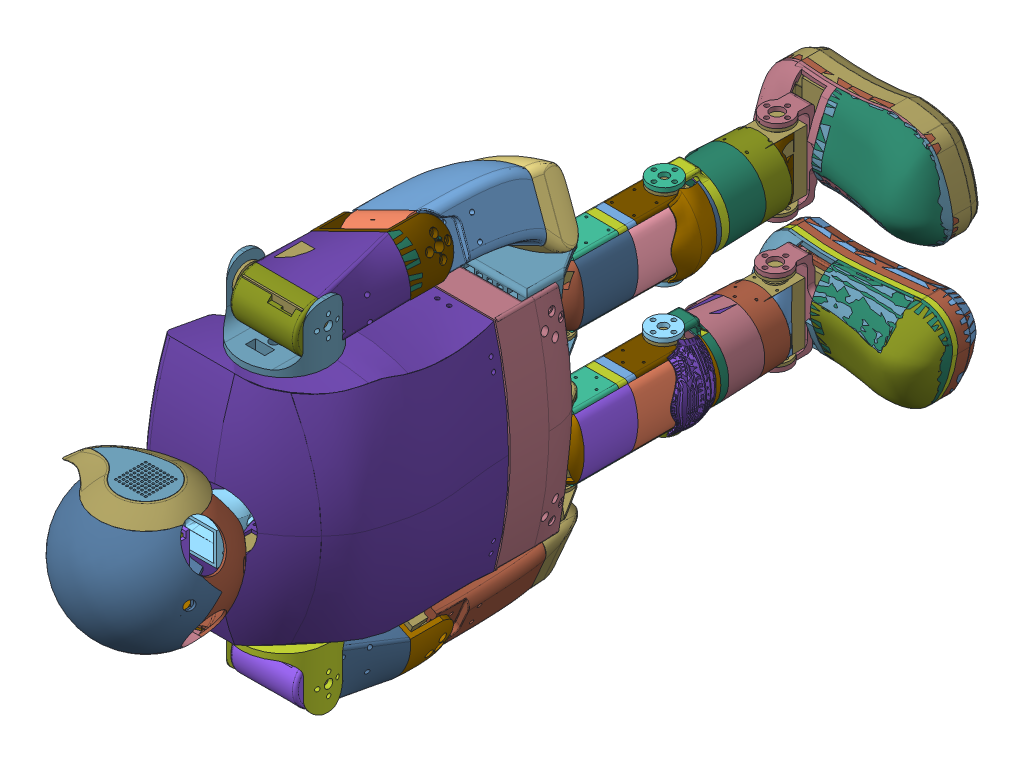
SolidWorks assembly ROBOT, configuration Default. Lengths in mm.
Overall size (168.02 284.66 497.18).
184 component instances, 104 part files, 132 mates.
Components (placement in the parent):
- right foot-1: right foot [Default] at (47.4769 97.6627 319.5854) size (123.36 70.36 23.98)
  - right foot-Part-1-1: right foot-Part-1 [默认] at (2.4797 75.1958 -228.2622) x (0 -1 0) z (0 0 1) size (70.36 123.36 10.26)
  - right foot-Part-2-1: right foot-Part-2 [默认] at (2.4797 75.1958 -228.2622) x (0 -1 0) z (0 0 1) size (5 5 3)
  - right foot-Part-3-1: right foot-Part-3 [默认] at (2.4797 75.1958 -228.2622) x (0 -1 0) z (0 0 1) size (5 5 3)
  - right foot-Part-4-1: right foot-Part-4 [默认] at (2.4797 75.1958 -228.2622) x (0 -1 0) z (0 0 1) size (5 5 3)
  - right foot-Part-5-1: right foot-Part-5 [默认] at (2.4797 75.1958 -228.2622) x (0 -1 0) z (0 0 1) size (3 3 3)
  - right foot-Part-6-1: right foot-Part-6 [默认] at (2.4797 75.1958 -228.2622) x (0 -1 0) z (0 0 1) size (3 3 3)
  - right foot-Part-7-1: right foot-Part-7 [默认] at (2.4797 75.1958 -228.2622) x (0 -1 0) z (0 0 1) size (68.42 123.23 13.95)
  - right foot-Part-8-1: right foot-Part-8 [默认] at (2.4797 75.1958 -228.2622) x (0 -1 0) z (0 0 1) size (3 3 3)
  - right foot-Part-9-1: right foot-Part-9 [默认] at (2.4797 75.1958 -228.2622) x (0 -1 0) z (0 0 1) size (5 5 3)
  - right foot-Part-10-1: right foot-Part-10 [默认] at (2.4797 75.1958 -228.2622) x (0 -1 0) z (0 0 1) size (3 3 3)
  - right foot-Part-11-1: right foot-Part-11 [默认] at (2.4797 75.1958 -228.2622) x (0 -1 0) z (0 0 1) size (70.36 123.36 19.01)
- servo-1: servo [Default] at (64.0611 111.5585 116.4732) x (0 0 1) z (0 1 0) size (20 51.7 40)
  - servo-Part-1-1: servo-Part-1 [默认] at (-33.15 -9.3942 -72.6) x (0 0 1) z (1 0 0) size (40 51.7 20)
- zhijiao-1: zhijiao [Default] at (47.3569 97.6627 319.5854) size (59.38 57.38 56.66)
  - zhijiao-Part-1-1: zhijiao-Part-1 [默认] at (-38.15 -124.7042 -221.2622) x (0 -1 0) z (-1 0 0) size (57.38 56.66 59.38)
- right foot cover-1: right foot cover [Default] at (47.5769 97.6627 319.5854) size (124.44 71 32.97)
  - right foot cover-Part-1-1: right foot cover-Part-1 [默认] at (2.3797 137.8816 -227.2622) x (0 -1 0) z (0 0 1) size (71 123.7 31.71)
  - right foot cover-Part-2-1: right foot cover-Part-2 [默认] at (2.3797 137.8816 -227.2622) x (0 -1 0) z (0 0 1) size (65.9 77.18 26.11)
  - right foot cover-Part-3-1: right foot cover-Part-3 [默认] at (2.3797 137.8816 -227.2622) x (0 -1 0) z (0 0 1) size (65.83 76.7 26.08)
- servo-2: servo [Default] at (1.0324 97.7127 87.3987) x (-1 0 0.000575) z (-0.000575 0 -1) size (20 51.7 40)
  - servo-Part-1-1: servo-Part-1 [默认] at (-33.15 -9.3942 -72.6) x (0 0 1) z (1 0 0) size (40 51.7 20)
- shank right-1: shank right [Default] at (14.2241 -102.1815 159.9911) x (-0.000575 0 -1) z (1 0 -0.000575) size (92.37 57.6 51.33)
  - shank right-Part-1-1: shank right-Part-1 [默认] at origin size (25 48.39 47.26)
  - shank right-Part-2-1: shank right-Part-2 [默认] at origin size (18.05 46 46)
  - shank right-Part-3-1: shank right-Part-3 [默认] at origin size (23.16 40.51 12.38)
  - shank right-Part-4-1: shank right-Part-4 [默认] at origin size (3 2.5 26)
  - shank right-Part-5-1: shank right-Part-5 [默认] at origin size (3 2.5 26)
  - shank right-Part-6-1: shank right-Part-6 [默认] at origin size (3 2.5 26)
  - shank right-Part-7-1: shank right-Part-7 [默认] at origin size (20 2.9 20)
  - shank right-Part-8-1: shank right-Part-8 [默认] at origin size (20 2.9 20)
  - shank right-Part-9-1: shank right-Part-9 [默认] at origin size (14.44 57.6 31.5)
  - shank right-Part-10-1: shank right-Part-10 [默认] at origin size (31.11 53.53 20.13)
  - shank right-Part-11-1: shank right-Part-11 [默认] at origin size (5.05 44.63 15.49)
  - shank right-Part-12-1: shank right-Part-12 [默认] at origin size (23.29 40.51 12.38)
  - shank right-Part-13-1: shank right-Part-13 [默认] at origin size (18.05 46 46)
  - shank right-Part-14-1: shank right-Part-14 [默认] at origin size (3 2.5 26)
  - shank right-Part-15-1: shank right-Part-15 [默认] at origin size (25 48.39 47.26)
  - shank right-Part-16-1: shank right-Part-16 [默认] at origin size (14.32 43.75 29.27)
  - shank right-Part-17-1: shank right-Part-17 [默认] at origin size (14.44 57.6 31.5)
  - shank right-Part-18-1: shank right-Part-18 [默认] at origin size (20 2.9 20)
  - shank right-Part-19-1: shank right-Part-19 [默认] at origin size (31.11 53.53 20.13)
- servo-3: servo [Default] at (1.1 97.6627 162.3854) x (-1 0 0) z (0 0 -1) size (20 51.7 40)
  - servo-Part-1-1: servo-Part-1 [默认] at (-33.15 -9.3942 -72.6) x (0 0 1) z (1 0 0) size (40 51.7 20)
- thigh-1: thigh [Default] at (1.1 127.7685 319.5854) x (-1 0 0) z (0 0 1) size (38.49 44.5 95.37)
  - thigh-Part-1-1: thigh-Part-1 [默认] at (-13.15 39.5 -84.6) x (0 1 0) z (0 0 1) size (44.5 24 30)
  - thigh-Part-2-1: thigh-Part-2 [默认] at (-13.15 39.5 -84.6) x (0 1 0) z (0 0 1) size (44.5 24 6)
  - thigh-Part-3-1: thigh-Part-3 [默认] at (-13.15 39.5 -84.6) x (0 1 0) z (0 0 1) size (40.5 9.43 36)
  - thigh-Part-4-1: thigh-Part-4 [默认] at (-13.15 39.5 -84.6) x (0 1 0) z (0 0 1) size (40.51 12.57 12)
  - thigh-Part-5-1: thigh-Part-5 [默认] at (-13.15 39.5 -84.6) x (0 1 0) z (0 0 1) size (40.5 9.43 36)
  - thigh-Part-6-1: thigh-Part-6 [默认] at (-13.15 39.5 -84.6) x (0 1 0) z (0 0 1) size (40.51 12.57 12.08)
  - thigh-Part-7-1: thigh-Part-7 [默认] at (-13.15 39.5 -84.6) x (0 1 0) z (0 0 1) size (44.5 24 30)
  - thigh-Part-8-1: thigh-Part-8 [默认] at (-13.15 39.5 -84.6) x (0 1 0) z (0 0 1) size (44.5 24 6)
  - thigh-Part-9-1: thigh-Part-9 [默认] at (-13.15 39.5 -84.6) x (0 1 0) z (0 0 1) size (40.5 9.43 36)
  - thigh-Part-10-1: thigh-Part-10 [默认] at (-13.15 39.5 -84.6) x (0 1 0) z (0 0 1) size (40.51 12.57 12.08)
  - thigh-Part-11-1: thigh-Part-11 [默认] at (-13.15 39.5 -84.6) x (0 1 0) z (0 0 1) size (40.5 9.43 36)
  - thigh-Part-12-1: thigh-Part-12 [默认] at (-13.15 39.5 -84.6) x (0 1 0) z (0 0 1) size (40.51 12.57 11.4)
- servo-4: servo [Default] at (47.4 97.6627 319.5854) size (20 51.7 40)
  - servo-Part-1-1: servo-Part-1 [默认] at (-33.15 -9.3942 -72.6) x (0 0 1) z (1 0 0) size (40 51.7 20)
- bottom right-1: bottom right [Default] at (47.4 97.6627 319.5854) size (44.79 57.7 52.6)
  - bottom right-Part-1-1: bottom right-Part-1 [默认] at (-42.5 42.9558 -20) size (44.79 57.7 52.6)
- servo-5: servo [Default] at (-4.4942 16.3185 332.7354) x (0 0 1) z (0 -1 0) size (20 51.7 40)
  - servo-Part-1-1: servo-Part-1 [默认] at (-33.15 -9.3942 -72.6) x (0 0 1) z (1 0 0) size (40 51.7 20)
- buttocks-1: buttocks [Default] at (47.4 97.6627 319.5854) size (72.1 145.63 51.57)
- servo-6: servo [Default] at (-4.4942 209.1127 286.4354) x (0 0 -1) z (0 1 0) size (20 51.7 40)
  - servo-Part-1-1: servo-Part-1 [默认] at (-33.15 -9.3942 -72.6) x (0 0 1) z (1 0 0) size (40 51.7 20)
- bottom left-2: bottom left [Default] at (47.4 97.6627 319.5854) size (44.75 57.7 52.6)
  - bottom left-Part-1-1: bottom left-Part-1 [默认] at (-42.5 38.85 -20) size (44.75 57.7 52.6)
- servo-8: servo [Default] at (0.7557 127.7685 319.3965) x (-0.999967 0 -0.0081) z (-0.0081 0 0.999967) size (20 51.7 40)
  - servo-Part-1-1: servo-Part-1 [默认] at (-33.15 -9.3942 -72.6) x (0 0 1) z (1 0 0) size (40 51.7 20)
- thigh-2: thigh [Default] at (47.0542 97.6627 319.7715) x (0.999967 0 0.0081) z (-0.0081 0 0.999967) size (38.49 44.5 95.37)
  - thigh-Part-1-1: thigh-Part-1 [默认] at (-13.15 39.5 -84.6) x (0 1 0) z (0 0 1) size (44.5 24 30)
  - thigh-Part-2-1: thigh-Part-2 [默认] at (-13.15 39.5 -84.6) x (0 1 0) z (0 0 1) size (44.5 24 6)
  - thigh-Part-3-1: thigh-Part-3 [默认] at (-13.15 39.5 -84.6) x (0 1 0) z (0 0 1) size (40.5 9.43 36)
  - thigh-Part-4-1: thigh-Part-4 [默认] at (-13.15 39.5 -84.6) x (0 1 0) z (0 0 1) size (40.51 12.57 12)
  - thigh-Part-5-1: thigh-Part-5 [默认] at (-13.15 39.5 -84.6) x (0 1 0) z (0 0 1) size (40.5 9.43 36)
  - thigh-Part-6-1: thigh-Part-6 [默认] at (-13.15 39.5 -84.6) x (0 1 0) z (0 0 1) size (40.51 12.57 12.08)
  - thigh-Part-7-1: thigh-Part-7 [默认] at (-13.15 39.5 -84.6) x (0 1 0) z (0 0 1) size (44.5 24 30)
  - thigh-Part-8-1: thigh-Part-8 [默认] at (-13.15 39.5 -84.6) x (0 1 0) z (0 0 1) size (44.5 24 6)
  - thigh-Part-9-1: thigh-Part-9 [默认] at (-13.15 39.5 -84.6) x (0 1 0) z (0 0 1) size (40.5 9.43 36)
  - thigh-Part-10-1: thigh-Part-10 [默认] at (-13.15 39.5 -84.6) x (0 1 0) z (0 0 1) size (40.51 12.57 12.08)
  - thigh-Part-11-1: thigh-Part-11 [默认] at (-13.15 39.5 -84.6) x (0 1 0) z (0 0 1) size (40.5 9.43 36)
  - thigh-Part-12-1: thigh-Part-12 [默认] at (-13.15 39.5 -84.6) x (0 1 0) z (0 0 1) size (40.51 12.57 11.4)
- servo-9: servo [Default] at (48.3275 127.7685 162.5766) x (0.999967 0 0.0081) z (0.0081 0 -0.999967) size (20 51.7 40)
  - servo-Part-1-1: servo-Part-1 [默认] at (-33.15 -9.3942 -72.6) x (0 0 1) z (1 0 0) size (40 51.7 20)
- shank left-1: shank left [Default] at (15.198 137.2127 159.9082) x (0.0081 0 -0.999967) z (0.999967 0 0.0081) size (92.37 57.6 51.33)
  - shank left-Part-1-1: shank left-Part-1 [默认] at origin size (25 48.39 47.26)
  - shank left-Part-2-1: shank left-Part-2 [默认] at origin size (18.05 46 46)
  - shank left-Part-3-1: shank left-Part-3 [默认] at origin size (23.29 40.51 12.38)
  - shank left-Part-4-1: shank left-Part-4 [默认] at origin size (23.16 40.51 12.38)
  - shank left-Part-5-1: shank left-Part-5 [默认] at origin size (3 2.5 26)
  - shank left-Part-6-1: shank left-Part-6 [默认] at origin size (3 2.5 26)
  - shank left-Part-7-1: shank left-Part-7 [默认] at origin size (3 2.5 26)
  - shank left-Part-8-1: shank left-Part-8 [默认] at origin size (3 2.5 26)
  - shank left-Part-9-1: shank left-Part-9 [默认] at origin size (20 2.9 20)
  - shank left-Part-10-1: shank left-Part-10 [默认] at origin size (20 2.9 20)
  - shank left-Part-11-1: shank left-Part-11 [默认] at origin size (14.44 57.6 31.5)
  - shank left-Part-12-1: shank left-Part-12 [默认] at origin size (14.32 43.75 29.27)
  - shank left-Part-13-1: shank left-Part-13 [默认] at origin size (31.11 53.53 20.13)
  - shank left-Part-14-1: shank left-Part-14 [默认] at origin size (5.05 44.63 15.49)
- servo-10: servo [Default] at (48.935 127.8185 87.5791) x (0.999967 0 0.0081) z (0.0081 0 -0.999967) size (20 51.7 40)
  - servo-Part-1-1: servo-Part-1 [默认] at (-33.15 -9.3942 -72.6) x (0 0 1) z (1 0 0) size (40 51.7 20)
- zhijiao-2: zhijiao [Default] at (47.0542 185.3769 319.7715) x (0.999967 0 0.0081) z (-0.0081 0 0.999967) size (59.38 57.38 56.66)
  - zhijiao-Part-1-1: zhijiao-Part-1 [默认] at (-38.15 -124.7042 -221.2622) x (0 -1 0) z (-1 0 0) size (57.38 56.66 59.38)
- servo-11: servo [Default] at (65.6579 114.0573 70.5301) x (0.0081 -0.000663 -0.999967) z (-0.000005 -1 0.000663) size (20 51.7 40)
  - servo-Part-1-1: servo-Part-1 [默认] at (-33.15 -9.3942 -72.6) x (0 0 1) z (1 0 0) size (40 51.7 20)
- left foot-1: left foot [Default] at (46.854 97.7127 319.809) x (0.999967 0 0.0081) z (-0.0081 0.000663 0.999967) size (123.36 70.36 28.78)
  - left foot-Part-1-1: left foot-Part-1 [默认] at (2.5796 67.11 -228.2622) x (0 -1 0) z (0 0 1) size (68.42 123.23 13.95)
  - left foot-Part-2-1: left foot-Part-2 [默认] at (2.5796 67.11 -228.2622) x (0 -1 0) z (0 0 1) size (70.36 123.36 28.78)
- left foot cover-1: left foot cover [Default] at (46.854 97.7127 319.809) x (0.999967 0 0.0081) z (-0.0081 0.000663 0.999967) size (124.44 71 32.97)
  - left foot cover-Part-1-1: left foot cover-Part-1 [默认] at (2.5796 67.11 -227.2622) x (0 -1 0) z (0 0 1) size (71 123.7 31.71)
  - left foot cover-Part-2-1: left foot cover-Part-2 [默认] at (2.5796 67.11 -227.2622) x (0 -1 0) z (0 0 1) size (65.9 77.18 26.11)
  - left foot cover-Part-3-1: left foot cover-Part-3 [默认] at (2.5796 67.11 -227.2622) x (0 -1 0) z (0 0 1) size (65.83 76.7 26.08)
- body_1-1: body_1 [Default] at (47.4 97.6627 320.5854) size (123.88 163.04 143.19)
  - body_1-Part-1-1: body_1-Part-1 [默认] at origin size (68.93 141.2 12)
  - body_1-Part-2-1: body_1-Part-2 [默认] at origin size (123.88 163.04 143.19)
  - body_1-Part-3-1: body_1-Part-3 [默认] at origin size (19 22 22)
  - body_1-Part-4-1: body_1-Part-4 [默认] at origin size (64.68 134 3)
  - body_1-Part-5-1: body_1-Part-5 [默认] at origin size (46.9 125.7 13.6)
  - body_1-Part-6-1: body_1-Part-6 [默认] at origin size (57.58 110.18 6.6)
  - body_1-Part-7-1: body_1-Part-7 [默认] at origin size (65 45 3)
  - body_1-Part-8-1: body_1-Part-8 [默认] at origin size (63.76 134 3)
- servo-12: servo [Default] at (66.85 135.8127 353.9796) x (0 1 0) z (1 0 0) size (20 51.7 40)
  - servo-Part-1-1: servo-Part-1 [默认] at (-33.15 -9.3942 -72.6) x (0 0 1) z (1 0 0) size (40 51.7 20)
- back batter-1: back batter [Default] at (47.3934 97.7627 320.4854) size (33.84 118.72 75.16)
- servo-13: servo [Default] at (24.9433 37.6156 393.9854) x (1 0 0) z (0 0 -1) size (20 51.7 40)
  - servo-Part-1-1: servo-Part-1 [默认] at (-33.15 -9.3942 -72.6) x (0 0 1) z (1 0 0) size (40 51.7 20)
- sholder righr-1: sholder righr [Default] at (47.3998 97.6627 320.5854) size (59.12 48 59.12)
  - sholder righr-Part-1-1: sholder righr-Part-1 [默认] at (-55.6065 -50.6528 146) x (0 0 -1) z (1 0 0) size (59.12 48 59.12)
- servo-14: servo [Default] at (-26.9509 31.9871 478.4187) x (0 0.999995 -0.00304) z (0 0.00304 0.999995) size (20 51.7 40)
  - servo-Part-1-1: servo-Part-1 [默认] at (-33.15 -9.3942 -72.6) x (0 0 1) z (1 0 0) size (40 51.7 20)
- shoulder right middle-1: shoulder right middle [Default] at (47.3998 99.5323 322.0523) x (1 0 0) z (0 -0.016318 0.999867) size (75.24 60.91 102.16)
  - shoulder right middle-Part-1-1: shoulder right middle-Part-1 [默认] at (-64.9565 -99.5338 85.5031) x (0 0.019357 0.999813) z (0 0.999813 -0.019357) size (16.5 44.5 33)
  - shoulder right middle-Part-2-1: shoulder right middle-Part-2 [默认] at (-64.9565 -99.5338 85.5031) x (0 0.019357 0.999813) z (0 0.999813 -0.019357) size (34.81 68.34 57.32)
  - shoulder right middle-Part-3-1: shoulder right middle-Part-3 [默认] at (-64.9565 -99.5338 85.5031) x (0 0.019357 0.999813) z (0 0.999813 -0.019357) size (50.4 75.24 59.94)
- servo-15: servo [Default] at (-15.4248 38.8821 407.356) x (0.440882 0.893064 0.089777) z (-0.040953 -0.079904 0.995961) size (20 51.7 40)
  - servo-Part-1-1: servo-Part-1 [默认] at (-33.15 -9.3942 -72.6) x (0 0 1) z (1 0 0) size (40 51.7 20)
- shoulder right end-1: shoulder right end [Default] at (48.8681 102.5348 331.6087) x (0.99916 -0.001577 0.040958) z (-0.040913 -0.099184 0.994228) size (72.21 68.93 79.01)
  - shoulder right end-Part-1-1: shoulder right end-Part-1 [默认] at (-64.9565 -99.5338 85.5031) x (0 0.019357 0.999813) z (0 0.999813 -0.019357) size (77.72 72.21 67.44)
- hand right-1: hand right [Default] at (48.8371 102.5503 331.6087) x (0.999159 -0.001237 0.040986) z (-0.040906 -0.099184 0.994228) size (72.22 67.73 36.31)
  - hand right-Part-1-1: hand right-Part-1 [默认] at (-64.9565 -99.5338 85.5031) x (0 0.019357 0.999813) z (0 0.999813 -0.019357) size (35.02 72.22 67.06)
- servo-16: servo [Default] at (-21.3565 187.7097 393.9854) x (-1 0 0) z (0 0 -1) size (20 51.7 40)
  - servo-Part-1-1: servo-Part-1 [默认] at (-33.15 -9.3942 -72.6) x (0 0 1) z (1 0 0) size (40 51.7 20)
- back of batter-1: back of batter [Default] at (47.3186 97.8627 320.4222) size (5.86 131.2 36.73)
- shoulder left-1: shoulder left [Default] at (47.4001 97.6627 320.5385) size (59.4 48 59.4)
  - shoulder left-Part-1-1: shoulder left-Part-1 [默认] at (-35.7474 80.6528 146.0935) x (0.00469 0 -0.999989) z (-0.999989 0 -0.00469) size (59.12 48 59.12)
- servo-17: servo [Default] at (-27.1469 239.7676 478.354) x (0 1 0) z (-0.00469 0 0.999989) size (20 51.7 40)
  - servo-Part-1-1: servo-Part-1 [默认] at (-33.15 -9.3942 -72.6) x (0 0 1) z (1 0 0) size (40 51.7 20)
- shoulder left_1-1: shoulder left_1 [Default] at (47.4003 93.7101 320.4897) x (1 0.000002 0) z (0 -0.00041 1) size (93.57 96.31 101.67)
  - shoulder left_1-Part-1-1: shoulder left_1-Part-1 [默认] at (13.0836 -28.7991 85.6863) x (-0.00469 0.00041 0.999989) z (-0.79401 0.607891 -0.003973) size (34.81 68.34 57.32)
  - shoulder left_1-Part-2-1: shoulder left_1-Part-2 [默认] at (13.0836 -28.7991 85.6863) x (-0.00469 0.00041 0.999989) z (-0.79401 0.607891 -0.003973) size (16.5 51.65 53.79)
  - shoulder left_1-Part-3-1: shoulder left_1-Part-3 [默认] at (13.0836 -28.7991 85.6863) x (-0.00469 0.00041 0.999989) z (-0.79401 0.607891 -0.003973) size (50.4 75.58 59.68)
  - shoulder left_1-Part-4-1: shoulder left_1-Part-4 [默认] at (13.0836 -28.7991 85.6863) x (-0.00469 0.00041 0.999989) z (-0.79401 0.607891 -0.003973) size (34.81 68.34 57.32)
- servo-18: servo [Default] at (-35.5113 223.348 403.2451) x (-0.440858 0.893535 -0.085085) z (-0.041431 0.074435 0.996365) size (20 51.7 40)
  - servo-Part-1-1: servo-Part-1 [默认] at (-33.15 -9.3942 -72.6) x (0 0 1) z (1 0 0) size (40 51.7 20)
- shouler left end-1: shouler left end [Default] at (48.724 90.9288 331.1172) x (0.999323 0.001023 0.036771) z (-0.036746 0.074031 0.996579) size (96.59 96.94 90.92)
  - shouler left end-Part-1-1: shouler left end-Part-1 [默认] at (13.0836 -28.7991 85.6863) x (-0.00469 0.00041 0.999989) z (-0.79401 0.607891 -0.003973) size (77.72 70.73 67.03)
  - shouler left end-Part-2-1: shouler left end-Part-2 [默认] at (13.0836 -28.7991 85.6863) x (-0.00469 0.00041 0.999989) z (-0.79401 0.607891 -0.003973) size (18 55.84 51.98)
- hand-1: hand [Default] at (48.7249 90.9291 331.1172) x (0.999323 0.001031 0.03677) z (-0.036746 0.074031 0.996579) size (96.37 96.7 35.47)
  - hand-Part-1-1: hand-Part-1 [默认] at (13.0836 -28.7991 85.6863) x (-0.00469 0.00041 0.999989) z (-0.79401 0.607891 -0.003973) size (35.02 70.08 67.52)
- little servo-1: little servo [Default] at (-190.3644 96.8207 388.5814) x (0.000015 -0.003813 -0.999993) z (0.999993 0.003813 0) size (29.47 32.61 17.8)
  - little servo-Part-1-1: little servo-Part-1 [默认] at (-43.0844 20.9951 186.1619) x (0.003813 -0.999993 0) z (-0.999993 -0.003813 0) size (32.5 17.8 29.35)
- neck_2-1: neck_2 [Default] at (47.4 97.6627 320.5854) size (35.1 22.14 38.58)
  - neck_2-Part-1-1: neck_2-Part-1 [默认] at (-51.6845 21.0269 111) x (0.003813 -0.999993 0) z (0 0 1) size (22.01 35.02 38.58)
- neck_1-1: neck_1 [Default] at (47.3999 97.6877 320.5854) size (11.37 17.84 30.21)
  - neck_1-Part-1-1: neck_1-Part-1 [默认] at (-49.1113 14.9471 205.3119) x (0.003813 -0.999993 0) z (0 0 1) size (17.8 11.3 30.21)
- neck_3-1: neck_3 [Default] at (47.3999 97.6877 320.5854) size (34.12 34.1 30.9)
  - neck_3-Part-1-1: neck_3-Part-1 [默认] at (-43.0844 20.9951 186.1619) x (0.003813 -0.999993 0) z (-0.999993 -0.003813 0) size (32.5 17.8 29.35)
  - neck_3-Part-1-2: neck_3-Part-1 [默认] at (-43.0844 20.9951 211.3619) x (-0.999993 -0.003813 0) z (0.003813 -0.999993 0) size (32.5 17.8 29.35)
  - neck_3-Part-2-1: neck_3-Part-2 [默认] at (-43.0844 20.9951 211.3619) x (-0.999993 -0.003813 0) z (0.003813 -0.999993 0) size (32.5 29.2 27.21)
- middle head-1: middle head [Default] at (47.3999 97.6877 320.5854) size (50.8 71.19 56.42)
  - middle head-Part-1-1: middle head-Part-1 [默认] at (-49.1113 14.9471 205.3119) x (0.003813 -0.999993 0) z (0 0 1) size (71 50.53 56.42)
- face_1-1: face_1 [Default] at (47.4003 97.5877 320.5854) size (95.35 92.36 93.5)
  - face_1-Part-1-1: face_1-Part-1 [默认] at (-49.1113 14.9471 205.3119) x (0.003813 -0.999993 0) z (0 0 1) size (92 95 93.5)
- face-1: face [Default] at (47.4003 97.5877 320.5854) size (30.47 73.52 50.7)
  - face-Part-1-1: face-Part-1 [默认] at (-49.1113 14.9471 205.3119) x (0.003813 -0.999993 0) z (0 0 1) size (73.4 30.19 50.7)
- ear left-1: ear left [Default] at (47.3999 97.6877 320.5854) size (82.76 15.37 65.48)
  - ear left-Part-1-1: ear left-Part-1 [默认] at (-49.1113 14.9471 205.3119) x (0.003813 -0.999993 0) z (0 0 1) size (15.05 82.7 65.48)
- ear right_1-1: ear right_1 [Default] at (47.3999 97.6877 320.5854) size (82.76 15.37 65.48)
  - ear right_1-Part-1-1: ear right_1-Part-1 [默认] at (-49.1113 14.9471 205.3119) x (0.003813 -0.999993 0) z (0 0 1) size (15.05 82.7 65.48)
- ear left_2-1: ear left_2 [Default] at (47.3999 97.6877 320.5854) size (54.62 2.22 38.67)
  - ear left_2-Part-1-1: ear left_2-Part-1 [默认] at (-49.1113 14.9471 205.3119) x (0.003813 -0.999993 0) z (0 0 1) size (2.01 54.62 38.67)
- ear left_2-2: ear left_2 [Default] at (47.724 12.6883 320.5854) size (54.62 2.22 38.67)
  - ear left_2-Part-1-1: ear left_2-Part-1 [默认] at (-49.1113 14.9471 205.3119) x (0.003813 -0.999993 0) z (0 0 1) size (2.01 54.62 38.67)
Mates (geometry in assembly coordinates):
- 重合1: coincident anti-aligned: plane of right foot-1/right foot-Part-11-1 through (49.9566 60.8585 83.3232) normal (0 0 1); plane of servo-1/servo-Part-1-1 through (54.6669 38.9585 83.3232) normal (0 0 -1)
- 重合2: coincident anti-aligned: plane of right foot-1/right foot-Part-11-1 through (49.9566 38.9585 91.3232) normal (0 1 0); plane of servo-1/servo-Part-1-1 through (14.1669 38.9585 103.3232) normal (0 -1 0)
- 重合3: coincident anti-aligned: plane of right foot-1/right foot-Part-11-1 through (54.6669 172.8585 91.3232) normal (-1 0 0); plane of servo-1/servo-Part-1-1 through (54.6669 38.9585 103.3232) normal (1 0 0)
- 重合4: coincident anti-aligned: plane of servo-1/servo-Part-1-1 through (9.4669 68.9585 93.3232) normal (-1 0 0); plane of zhijiao-1/zhijiao-Part-1-1 through (9.4669 68.9585 93.3232) normal (1 0 0)
- 同心1: concentric anti-aligned: circle of servo-1/servo-Part-1-1; cylinder of zhijiao-1/zhijiao-Part-1-1 through (5.2069 68.9585 93.3232) axis (1 0 0) radius 4.5
- 同心11: concentric aligned: cylinder of right foot-1/right foot-Part-7-1 through (37.5557 80.5578 96.3232) axis (0 0 1) radius 74.6364; cylinder of right foot cover-1/right foot cover-Part-1-1 through (37.5557 80.5578 98.3232) axis (0 0 1) radius 74.5364
- 重合10: coincident aligned: plane of right foot-1/right foot-Part-7-1 through (-10.1967 55.6363 96.3232) normal (-1 0 0); plane of right foot cover-1/right foot cover-Part-1-1 through (-10.1967 71.5793 100.3232) normal (-1 0 0)
- 重合12: coincident anti-aligned: plane of zhijiao-1/zhijiao-Part-1-1 through (24.2069 43.1185 129.9854) normal (0 1 0); plane of servo-2/servo-Part-1-1 through (24.2069 43.1185 129.9854) normal (0 -1 0)
- 同心13: concentric aligned: cylinder of zhijiao-1/zhijiao-Part-1-1 through (24.2069 42.8585 129.9854) axis (0 -1 0) radius 4.5; circle of servo-2/servo-Part-1-1
- 重合13: coincident anti-aligned: plane of servo-2/servo-Part-1-1 through (34.2241 88.3185 159.9796) normal (1 0 -0.000575); plane of shank right-1/shank right-Part-13-1 through (34.2241 88.3185 159.9796) normal (-1 0 0.000575)
- 重合14: coincident anti-aligned: plane of servo-2/servo-Part-1-1 through (14.2241 47.8185 159.9911) normal (0.000575 0 1); plane of shank right-1/shank right-Part-6-1 through (14.2241 88.3185 159.9911) normal (-0.000575 0 -1)
- 重合15: coincident anti-aligned: plane of servo-2/servo-Part-1-1 through (14.2241 88.3185 159.9911) normal (0 1 0); plane of shank right-1/shank right-Part-13-1 through (34.2241 88.3185 159.9796) normal (0 -1 0)
- 重合16: coincident anti-aligned: plane of shank right-1/shank right-Part-18-1 through (27.75 43.0685 204.9834) normal (0 1 0); plane of servo-3/servo-Part-1-1 through (24.25 43.0685 204.9854) normal (0 -1 0)
- 同心16: concentric aligned: cylinder of shank right-1/shank right-Part-7-1 through (24.25 98.0585 204.9854) axis (0 -1 0) radius 3.1; circle of servo-3/servo-Part-1-1
- 重合17: coincident anti-aligned: plane of servo-3/servo-Part-1-1 through (34.25 88.2685 234.9854) normal (1 0 0); plane of thigh-1/thigh-Part-1-1 through (34.25 47.7685 204.9854) normal (-1 0 0)
- 重合18: coincident anti-aligned: plane of servo-3/servo-Part-1-1 through (14.25 47.7685 234.9854) normal (0 0 1); plane of thigh-1/thigh-Part-2-1 through (14.25 88.2685 234.9854) normal (0 0 -1)
- 重合19: coincident anti-aligned: plane of servo-3/servo-Part-1-1 through (14.25 47.7685 194.9854) normal (0 -1 0); plane of thigh-1/thigh-Part-1-1 through (14.25 47.7685 204.9854) normal (0 1 0)
- 重合20: coincident anti-aligned: plane of thigh-1/thigh-Part-7-1 through (14.25 88.2685 276.9854) normal (1 0 0); plane of servo-4/servo-Part-1-1 through (14.25 88.2685 246.9854) normal (-1 0 0)
- 重合21: coincident anti-aligned: plane of thigh-1/thigh-Part-7-1 through (34.25 88.2685 276.9854) normal (0 -1 0); plane of servo-4/servo-Part-1-1 through (34.25 88.2685 246.9854) normal (0 1 0)
- 重合22: coincident anti-aligned: plane of thigh-1/thigh-Part-8-1 through (14.25 88.2685 246.9854) normal (0 0 1); plane of servo-4/servo-Part-1-1 through (34.25 47.7685 246.9854) normal (0 0 -1)
- 重合33: coincident anti-aligned: plane of servo-4/servo-Part-1-1 through (24.25 43.0685 276.9854) normal (0 -1 0); plane of bottom right-1/bottom right-Part-1-1 through (24.25 43.0685 276.9854) normal (0 1 0)
- 同心25: concentric anti-aligned: circle of servo-4/servo-Part-1-1; cylinder of bottom right-1/bottom right-Part-1-1 through (24.25 40.0685 276.9854) axis (0 1 0) radius 3
- 重合34: coincident anti-aligned: plane of bottom right-1/bottom right-Part-1-1 through (4.9 88.9185 299.5854) normal (0 0 1); plane of servo-5/servo-Part-1-1 through (4.9 88.9185 299.5854) normal (0 0 -1)
- 重合35: coincident anti-aligned: plane of bottom right-1/bottom right-Part-1-1 through (45.4 48.9185 299.5854) normal (0 1 0); plane of servo-5/servo-Part-1-1 through (4.9 48.9185 319.5854) normal (0 -1 0)
- 重合37: coincident anti-aligned: plane of servo-5/servo-Part-1-1 through (-1.6 58.9185 309.5854) normal (-1 0 0); plane of buttocks-1 through (-1.6 112.6627 603.606) normal (1 0 0)
- 同心27: concentric anti-aligned: circle of servo-5/servo-Part-1-1; cylinder of buttocks-1 through (-1.2 58.9185 309.5854) axis (-1 0 0) radius 3.1
- 重合38: coincident anti-aligned: plane of buttocks-1 through (-1.6 112.6627 603.606) normal (1 0 0); plane of servo-6/servo-Part-1-1 through (-1.6 166.5127 309.5854) normal (-1 0 0)
- 同心29: concentric anti-aligned: cylinder of buttocks-1 through (-1.2 166.5127 309.5854) axis (-1 0 0) radius 3.1; circle of servo-6/servo-Part-1-1
- 重合39: coincident anti-aligned: plane of servo-6/servo-Part-1-1 through (45.4 136.5127 299.5854) normal (0 -1 0); plane of bottom left-2/bottom left-Part-1-1 through (4.9 136.5127 299.5854) normal (0 1 0)
- 重合40: coincident anti-aligned: plane of servo-6/servo-Part-1-1 through (45.4 176.5127 299.5854) normal (1 0 0); plane of bottom left-2/bottom left-Part-1-1 through (45.4 136.5127 299.5854) normal (-1 0 0)
- 重合41: coincident anti-aligned: plane of servo-6/servo-Part-1-1 through (4.9 136.5127 299.5854) normal (0 0 -1); plane of bottom left-2/bottom left-Part-1-1 through (4.9 136.5127 299.5854) normal (0 0 1)
- 重合42: coincident anti-aligned: plane of bottom left-2/bottom left-Part-1-1 through (24.25 130.6627 276.9854) normal (0 1 0); plane of servo-8/servo-Part-1-1 through (24.25 130.6627 276.9854) normal (0 -1 0)
- 同心31: concentric aligned: cylinder of bottom left-2/bottom left-Part-1-1 through (24.25 127.6627 276.9854) axis (0 1 0) radius 3; circle of servo-8/servo-Part-1-1
- 重合43: coincident anti-aligned: plane of servo-8/servo-Part-1-1 through (14.4933 137.1627 246.9054) normal (-0.999967 0 -0.0081); plane of thigh-2/thigh-Part-7-1 through (14.2503 177.6627 276.9044) normal (0.999967 0 0.0081)
- 重合44: coincident anti-aligned: plane of servo-8/servo-Part-1-1 through (14.4933 177.6627 246.9054) normal (0.0081 0 -0.999967); plane of thigh-2/thigh-Part-8-1 through (34.4927 137.1627 247.0674) normal (-0.0081 0 0.999967)
- 重合45: coincident anti-aligned: plane of servo-8/servo-Part-1-1 through (14.1693 177.6627 286.904) normal (0 1 0); plane of thigh-2/thigh-Part-7-1 through (34.2497 177.6627 277.0664) normal (0 -1 0)
- 重合46: coincident anti-aligned: plane of thigh-2/thigh-Part-1-1 through (14.8335 177.6627 204.9067) normal (0.999967 0 0.0081); plane of servo-9/servo-Part-1-1 through (14.5905 137.1627 234.9057) normal (-0.999967 0 -0.0081)
- 重合47: coincident anti-aligned: plane of thigh-2/thigh-Part-2-1 through (34.5899 137.1627 235.0678) normal (0.0081 0 -0.999967); plane of servo-9/servo-Part-1-1 through (34.5899 177.6627 235.0678) normal (-0.0081 0 0.999967)
- 重合48: coincident anti-aligned: plane of thigh-2/thigh-Part-1-1 through (14.8335 137.1627 204.9067) normal (0 1 0); plane of servo-9/servo-Part-1-1 through (34.5899 137.1627 235.0678) normal (0 -1 0)
- 同心33: concentric aligned: circle of servo-9/servo-Part-1-1; cylinder of shank left-1/shank left-Part-9-1 through (24.8332 127.4727 204.9877) axis (0 1 0) radius 3.1
- 重合49: coincident anti-aligned: plane of servo-9/servo-Part-1-1 through (24.8332 130.6627 204.9877) normal (0 -1 0); plane of shank left-1/shank left-Part-9-1 through (24.8616 130.6627 201.4878) normal (0 1 0)
- 重合50: coincident anti-aligned: plane of shank left-1/shank left-Part-2-1 through (35.1974 137.2127 160.0702) normal (0 1 0); plane of servo-10/servo-Part-1-1 through (35.1974 137.2127 160.0702) normal (0 -1 0)
- 重合51: coincident anti-aligned: plane of shank left-1/shank left-Part-8-1 through (15.198 137.2127 159.9082) normal (0.0081 0 -0.999967); plane of servo-10/servo-Part-1-1 through (35.1974 177.7127 160.0702) normal (-0.0081 0 0.999967)
- 重合52: coincident anti-aligned: plane of shank left-1/shank left-Part-2-1 through (35.1974 137.2127 160.0702) normal (-0.999967 0 -0.0081); plane of servo-10/servo-Part-1-1 through (35.1974 137.2127 160.0702) normal (0.999967 0 0.0081)
- 重合53: coincident anti-aligned: plane of servo-10/servo-Part-1-1 through (25.4407 182.4127 129.9902) normal (0 1 0); plane of zhijiao-2/zhijiao-Part-1-1 through (25.4407 182.4127 129.9902) normal (0 -1 0)
- 同心34: concentric aligned: circle of servo-10/servo-Part-1-1; cylinder of zhijiao-2/zhijiao-Part-1-1 through (25.4407 182.4127 129.9902) axis (0 1 0) radius 4.5
- 重合56: coincident anti-aligned: plane of zhijiao-2/zhijiao-Part-1-1 through (62.5765 156.6727 93.6276) normal (-0.999967 0 -0.0081); plane of servo-11/servo-Part-1-1 through (62.5765 156.6727 93.6276) normal (0.999967 0 0.0081)
- 同心38: concentric anti-aligned: cylinder of zhijiao-2/zhijiao-Part-1-1 through (62.5765 156.6727 93.6276) axis (0.999967 0 0.0081) radius 4.5; circle of servo-11/servo-Part-1-1
- 重合57: coincident anti-aligned: plane of servo-11/servo-Part-1-1 through (56.1576 146.666 83.5819) normal (-0.000005 -1 0.000663); plane of left foot-1/left foot-Part-2-1 through (15.6347 146.668 86.2538) normal (0.000005 1 -0.000663)
- 重合58: coincident anti-aligned: plane of servo-11/servo-Part-1-1 through (15.659 146.666 83.2539) normal (-0.999967 0 -0.0081); plane of left foot-1/left foot-Part-2-1 through (15.6349 186.668 86.2273) normal (0.999967 0 0.0081)
- 重合59: coincident anti-aligned: plane of servo-11/servo-Part-1-1 through (56.1578 186.666 83.5554) normal (0.0081 -0.000663 -0.999967); plane of left foot-1/left foot-Part-2-1 through (51.3476 164.666 83.531) normal (-0.0081 0.000663 0.999967)
- 重合60: coincident anti-aligned: plane of left foot-1/left foot-Part-1-1 through (71.3395 125.6523 100.7194) normal (-0.0081 0.000663 0.999967); plane of left foot cover-1/left foot cover-Part-1-1 through (50.0729 134.8079 100.5411) normal (0.0081 -0.000663 -0.999967)
- 同心40: concentric aligned: cylinder of left foot-1/left foot-Part-1-1 through (14.6268 169.8968 96.2305) axis (-0.0081 0.000663 0.999967) radius 22.5366; cylinder of left foot cover-1/left foot cover-Part-1-1 through (14.6106 169.8981 98.2305) axis (-0.0081 0.000663 0.999967) radius 22.4366
- 重合61: coincident aligned: plane of left foot-1/left foot-Part-1-1 through (-8.909 169.8968 96.0399) normal (-0.999967 0 -0.0081); plane of left foot cover-1/left foot cover-Part-1-1 through (-8.9415 153.9565 100.0503) normal (-0.999967 0 -0.0081)
- 重合62: coincident anti-aligned: plane of bottom right-1/bottom right-Part-1-1 through (4.9 48.9185 299.5854) normal (1 0 0); plane of servo-5/servo-Part-1-1 through (4.9 88.9185 319.5854) normal (-1 0 0)
- 重合64: coincident anti-aligned: plane of buttocks-1 through (1.4 102.6627 345.5854) normal (0 1 0); plane of servo-12/servo-Part-1-1 through (-5.75 102.6627 344.5854) normal (0 -1 0)
- 重合65: coincident anti-aligned: plane of buttocks-1 through (47.4 97.6627 304.0854) normal (0 0 1); plane of servo-12/servo-Part-1-1 through (34.25 122.6627 304.0854) normal (0 0 -1)
- 重合66: coincident anti-aligned: plane of buttocks-1 through (34.25 102.6627 304.0854) normal (-1 0 0); plane of servo-12/servo-Part-1-1 through (34.25 122.6627 344.5854) normal (1 0 0)
- 重合67: coincident anti-aligned: plane of body_1-1/body_1-Part-1-1 through (24.25 112.6627 351.0854) normal (0 0 -1); plane of servo-12/servo-Part-1-1 through (24.25 112.6627 351.0854) normal (0 0 1)
- 同心47: concentric anti-aligned: cylinder of body_1-1/body_1-Part-1-1 through (24.25 112.6627 351.9854) axis (0 0 1) radius 4; circle of servo-12/servo-Part-1-1
- 重合68: coincident anti-aligned: plane of body_1-1/body_1-Part-2-1 through (-2.6 155.3627 354.4854) normal (0 0 1); plane of back batter-1 through (-2.6066 155.4627 354.4854) normal (0 0 -1)
- 重合70: coincident anti-aligned: plane of body_1-1/body_1-Part-2-1 through (-2.6 155.4627 411.5854) normal (0 -1 0); plane of back batter-1 through (-2.6066 155.4627 411.4854) normal (0 1 0)
- 锁定1: lock: unknown of ?; unknown of back batter-1
- 重合74: coincident anti-aligned: plane of body_1-1/body_1-Part-2-1 through (47.4 127.6627 466.5854) normal (0 0 -1); plane of servo-13/servo-Part-1-1 through (11.7933 87.5098 466.5854) normal (0 0 1)
- 重合75: coincident anti-aligned: plane of body_1-1/body_1-Part-2-1 through (11.7933 87.5098 436.5854) normal (-1 0 0); plane of servo-13/servo-Part-1-1 through (11.7933 47.0098 466.5854) normal (1 0 0)
- 重合76: coincident anti-aligned: plane of body_1-1/body_1-Part-2-1 through (-8.2065 87.5098 436.5854) normal (0 -1 0); plane of servo-13/servo-Part-1-1 through (11.7933 87.5098 426.5854) normal (0 1 0)
- 重合77: coincident anti-aligned: plane of servo-13/servo-Part-1-1 through (1.7933 40.5098 436.5854) normal (0 -1 0); plane of sholder righr-1/sholder righr-Part-1-1 through (1.7933 40.5098 433.0854) normal (0 1 0)
- 同心48: concentric aligned: circle of servo-13/servo-Part-1-1; cylinder of sholder righr-1/sholder righr-Part-1-1 through (1.7933 32.5098 436.5854) axis (0 1 0) radius 3.5
- 重合78: coincident anti-aligned: plane of sholder righr-1/sholder righr-Part-1-1 through (-24.0567 -7.4902 449.7299) normal (1 0 0); plane of servo-14/servo-Part-1-1 through (-24.0567 8.7077 435.8893) normal (-1 0 0)
- 同心49: concentric aligned: cylinder of sholder righr-1/sholder righr-Part-1-1 through (-38.8567 8.7077 435.8893) axis (1 0 0) radius 2.9; circle of servo-14/servo-Part-1-1
- 重合81: coincident anti-aligned: plane of servo-14/servo-Part-1-1 through (-17.5567 18.6165 405.859) normal (0 0.999995 -0.00304); plane of shoulder right middle-1/shoulder right middle-Part-3-1 through (22.9433 18.6165 405.859) normal (0 -0.999995 0.00304)
- 重合82: coincident anti-aligned: plane of servo-14/servo-Part-1-1 through (22.9433 18.6165 405.859) normal (0 -0.00304 -0.999995); plane of shoulder right middle-1/shoulder right middle-Part-3-1 through (-17.5567 -1.3834 405.9198) normal (0 0.00304 0.999995)
- 重合83: coincident anti-aligned: plane of servo-14/servo-Part-1-1 through (22.9433 18.738 445.8588) normal (1 0 0); plane of shoulder right middle-1/shoulder right middle-Part-3-1 through (22.9433 -1.3834 405.9198) normal (-1 0 0)
- 重合84: coincident anti-aligned: plane of shoulder right middle-1/shoulder right middle-Part-2-1 through (-21.2916 20.3301 362.8536) normal (0.89663 -0.442778 0.001346); plane of servo-15/servo-Part-1-1 through (-21.2916 20.3301 362.8536) normal (-0.89663 0.442778 -0.001346)
- 同心50: concentric aligned: cylinder of shoulder right middle-1/shoulder right middle-Part-2-1 through (-46.3972 32.7279 362.8159) axis (0.89663 -0.442778 0.001346) radius 3.25; circle of servo-15/servo-Part-1-1
- 重合85: coincident anti-aligned: plane of servo-15/servo-Part-1-1 through (24.8493 7.6511 373.7742) normal (0.89663 -0.442778 0.001346); plane of shoulder right end-1/shoulder right end-Part-1-1 through (26.4875 10.8473 333.9358) normal (-0.89663 0.442778 -0.001346)
- 重合86: coincident anti-aligned: plane of servo-15/servo-Part-1-1 through (-9.8261 28.7798 333.8813) normal (0.440882 0.893064 0.089777); plane of shoulder right end-1/shoulder right end-Part-1-1 through (-9.8261 28.7798 333.8813) normal (-0.440882 -0.893064 -0.089777)
- 重合87: coincident anti-aligned: plane of servo-15/servo-Part-1-1 through (26.4875 10.8473 333.9358) normal (0.040953 0.079904 -0.995961); plane of shoulder right end-1/shoulder right end-Part-1-1 through (-16.2941 0.9468 331.3824) normal (-0.040953 -0.079904 0.995961)
- 重合88: coincident aligned: cylinder of shoulder right end-1/shoulder right end-Part-1-1 through (4.4068 13.8026 301.8068) axis (0.040953 0.079904 -0.995961) radius 1.5; circle of hand right-1/hand right-Part-1-1
- 重合89: coincident anti-aligned: plane of shoulder right end-1/shoulder right end-Part-1-1 through (-2.9382 -1.0939 294.2853) normal (0.040953 0.079904 -0.995961); plane of hand right-1/hand right-Part-1-1 through (-2.9329 -1.0965 294.2853) normal (-0.040953 -0.079904 0.995961)
- 重合90: coincident anti-aligned: plane of body_1-1/body_1-Part-2-1 through (-8.2065 178.3155 436.5854) normal (1 0 0); plane of servo-16/servo-Part-1-1 through (-8.2065 178.3155 466.5854) normal (-1 0 0)
- 重合91: coincident anti-aligned: plane of body_1-1/body_1-Part-2-1 through (47.4 97.6627 466.5854) normal (0 0 -1); plane of servo-16/servo-Part-1-1 through (-8.2065 137.8155 466.5854) normal (0 0 1)
- 重合92: coincident anti-aligned: plane of body_1-1/body_1-Part-2-1 through (-8.2065 137.8155 436.5854) normal (0 1 0); plane of servo-16/servo-Part-1-1 through (-8.2065 137.8155 426.5854) normal (0 -1 0)
- 重合97: coincident anti-aligned: plane of body_1-1/body_1-Part-2-1 through (-32.6 168.3627 439.4854) normal (0 0 1); plane of back of batter-1 through (-44.6814 168.5627 439.4854) normal (0 0 -1)
- 重合98: coincident anti-aligned: plane of body_1-1/body_1-Part-2-1 through (-32.6 170.4627 471.5854) normal (0 -1 0); plane of back of batter-1 through (-44.6814 170.4627 471.3854) normal (0 1 0)
- 锁定5: lock: unknown of ?; unknown of back of batter-1
- 同心51: concentric aligned: circle of servo-16/servo-Part-1-1; cylinder of shoulder left-1/shoulder left-Part-1-1 through (1.7933 192.8155 436.5854) axis (0 -1 0) radius 3.5
- 重合99: coincident anti-aligned: plane of servo-16/servo-Part-1-1 through (1.7935 184.8155 436.5854) normal (0 1 0); plane of shoulder left-1/shoulder left-Part-1-1 through (1.8097 184.8155 433.0854) normal (0 -1 0)
- 重合100: coincident anti-aligned: plane of shoulder left-1/shoulder left-Part-1-1 through (-23.9948 232.8155 423.3198) normal (0.999989 0 0.00469); plane of servo-17/servo-Part-1-1 through (-24.0532 216.6176 435.768) normal (-0.999989 0 -0.00469)
- 同心52: concentric anti-aligned: cylinder of shoulder left-1/shoulder left-Part-1-1 through (42.4461 216.6176 436.0799) axis (-0.999989 0 -0.00469) radius 2.9; circle of servo-17/servo-Part-1-1
- 重合101: coincident anti-aligned: plane of servo-17/servo-Part-1-1 through (-17.4126 226.6176 405.7989) normal (-0.999989 0 -0.00469); plane of shoulder left_1-1/shoulder left_1-Part-3-1 through (-17.4126 202.6176 405.7989) normal (0.999989 0 0.00469)
- 重合102: coincident anti-aligned: plane of servo-17/servo-Part-1-1 through (23.087 226.6176 405.9888) normal (0.00469 0 -0.999989); plane of shoulder left_1-1/shoulder left_1-Part-3-1 through (-17.4126 222.6176 405.7989) normal (-0.00469 0 0.999989)
- 重合103: coincident anti-aligned: plane of servo-17/servo-Part-1-1 through (-17.4126 226.6176 405.7989) normal (0 1 0); plane of shoulder left_1-1/shoulder left_1-Part-3-1 through (10.4957 226.6176 425.43) normal (0 -1 0)
- 重合104: coincident anti-aligned: plane of shoulder left_1-1/shoulder left_1-Part-1-1 through (-20.9457 200.7732 362.7818) normal (0.89662 0.44278 0.004205); plane of servo-18/servo-Part-1-1 through (-20.9457 200.7732 362.7818) normal (-0.89662 -0.44278 -0.004205)
- 同心54: concentric aligned: cylinder of shoulder left_1-1/shoulder left_1-Part-1-1 through (-46.0511 188.3754 362.6641) axis (0.89662 0.44278 0.004205) radius 3.25; circle of servo-18/servo-Part-1-1
- 重合105: coincident anti-aligned: plane of servo-18/servo-Part-1-1 through (-18.2833 210.3536 332.0674) normal (-0.89662 -0.44278 -0.004205); plane of shouler left end-1/shouler left end-Part-1-1 through (-18.2833 210.3536 332.0674) normal (0.89662 0.44278 0.004205)
- 重合106: coincident anti-aligned: plane of servo-18/servo-Part-1-1 through (18.0298 228.2862 332.2377) normal (0.041431 -0.074435 -0.996365); plane of shouler left end-1/shouler left end-Part-1-1 through (-15.9336 220.3291 331.4198) normal (-0.041431 0.074435 0.996365)
- 重合107: coincident anti-aligned: plane of servo-18/servo-Part-1-1 through (-18.2833 210.3536 332.0674) normal (-0.440858 0.893535 -0.085085); plane of shouler left end-1/shouler left end-Part-1-1 through (18.0298 228.2862 332.2377) normal (0.440858 -0.893535 0.085085)
- 同心55: concentric anti-aligned: cylinder of shouler left end-1/shouler left end-Part-1-1 through (4.7817 207.6362 301.7841) axis (0.041431 -0.074435 -0.996365) radius 1.5; cylinder of hand-1/hand-Part-1-1 through (5.2789 206.743 289.8277) axis (-0.041431 0.074435 0.996365) radius 1.5
- 重合108: coincident anti-aligned: plane of shouler left end-1/shouler left end-Part-1-1 through (-2.56 222.5736 294.341) normal (0.041431 -0.074435 -0.996365); plane of hand-1/hand-Part-1-1 through (-2.5601 222.5736 294.341) normal (-0.041431 0.074435 0.996365)
- 重合109: coincident anti-aligned: plane of body_1-1/body_1-Part-2-1 through (7.8154 118.7357 439.5854) normal (-0.999993 -0.003813 0); plane of little servo-1/little servo-Part-1-1 through (7.9038 95.5258 452.8354) normal (0.999993 0.003813 0)
- 重合110: coincident anti-aligned: plane of body_1-1/body_1-Part-2-1 through (-4.2846 118.6895 439.5854) normal (0.003813 -0.999993 0); plane of little servo-1/little servo-Part-1-1 through (7.8154 118.7357 452.8354) normal (-0.003813 0.999993 0)
- 重合111: coincident anti-aligned: plane of body_1-1/body_1-Part-2-1 through (-6.4218 285.8365 448.3854) normal (0 0 1); plane of little servo-1/little servo-Part-1-1 through (-3.7523 123.3366 448.3854) normal (0 0 -1)
- 重合112: coincident anti-aligned: plane of little servo-1/little servo-Part-1-1 through (1.7885 112.6627 460.9354) normal (0 0 1); plane of neck_2-1/neck_2-Part-1-1 through (-1.7115 112.6493 460.9354) normal (0 0 -1)
- 同心56: concentric anti-aligned: circle of little servo-1/little servo-Part-1-1; cylinder of neck_2-1/neck_2-Part-1-1 through (1.7885 112.6627 464.9354) axis (0 0 -1) radius 3.5
- 同心57: concentric aligned: cylinder of neck_2-1/neck_2-Part-1-1 through (-17.396 108.5499 494.7154) axis (0.999993 0.003813 0) radius 0.9896; cylinder of neck_1-1/neck_1-Part-1-1 through (-19.696 108.5411 494.7154) axis (0.999993 0.003813 0) radius 1
- 平行1: parallel aligned: cylinder of neck_2-1/neck_2-Part-1-1 through (-17.4265 116.5498 494.7154) axis (0.999993 0.003813 0) radius 1; cylinder of neck_1-1/neck_1-Part-1-1 through (-19.7266 116.5661 494.7154) axis (0.999993 0.003813 0) radius 1
- 重合113: coincident anti-aligned: plane of neck_2-1/neck_2-Part-1-1 through (-15.6695 101.596 487.9354) normal (-0.999993 -0.003813 0); plane of neck_1-1/neck_1-Part-1-1 through (-15.7113 112.5814 525.8972) normal (0.999993 0.003813 0)
- 同心59: concentric aligned: cylinder of neck_1-1/neck_1-Part-1-1 through (-25.0112 112.5209 512.7972) axis (-0.999993 -0.003813 0) radius 3.5; circle of neck_3-1/neck_3-Part-1-1
- 重合114: coincident anti-aligned: plane of neck_1-1/neck_1-Part-1-1 through (-25.0112 112.5209 512.7972) normal (0.999993 0.003813 0); plane of neck_3-1/neck_3-Part-1-1 through (-25.0112 112.5209 512.7972) normal (-0.999993 -0.003813 0)
- 同心60: concentric aligned: circle of neck_3-1/neck_3-Part-1-2; cylinder of middle head-1/middle head-Part-1-1 through (-1.6225 89.3099 525.8972) axis (0.003813 -0.999993 0) radius 3.5
- 重合115: coincident anti-aligned: plane of neck_3-1/neck_3-Part-1-2 through (-1.6225 89.3099 525.8972) normal (0.003813 -0.999993 0); plane of middle head-1/middle head-Part-1-1 through (-1.6225 89.3099 525.8972) normal (-0.003813 0.999993 0)
- 重合116: coincident anti-aligned: plane of middle head-1/middle head-Part-1-1 through (-1.5818 78.635 525.8972) normal (-0.003813 0.999993 0); plane of face_1-1/face_1-Part-1-1 through (-1.5818 78.635 525.8972) normal (0.003813 -0.999993 0)
- 同心61: concentric aligned: cylinder of middle head-1/middle head-Part-1-1 through (-16.6301 78.5776 504.7481) axis (0.003813 -0.999993 0) radius 1; cylinder of face_1-1/face_1-Part-1-1 through (-16.6354 79.9776 504.7481) axis (0.003813 -0.999993 0) radius 1
- 同心62: concentric aligned: cylinder of middle head-1/middle head-Part-1-1 through (20.3177 148.219 539.4217) axis (0.003813 -0.999993 0) radius 1; cylinder of face_1-1/face_1-Part-1-1 through (20.575 80.7195 539.4217) axis (0.003813 -0.999993 0) radius 1
- 重合117: coincident anti-aligned: plane of middle head-1/middle head-Part-1-1 through (-1.5818 78.635 525.8972) normal (-0.003813 0.999993 0); plane of face-1/face-Part-1-1 through (-1.5818 78.635 525.8972) normal (0.003813 -0.999993 0)
- 同心63: concentric aligned: cylinder of middle head-1/middle head-Part-1-1 through (22.0499 78.7251 515.1608) axis (0.003813 -0.999993 0) radius 1; cylinder of face-1/face-Part-1-1 through (22.0446 80.1251 515.1608) axis (0.003813 -0.999993 0) radius 1
- 同心64: concentric aligned: cylinder of middle head-1/middle head-Part-1-1 through (19.8266 78.7166 511.2203) axis (0.003813 -0.999993 0) radius 1; cylinder of face-1/face-Part-1-1 through (19.8212 80.1166 511.2203) axis (0.003813 -0.999993 0) radius 1
- 同心65: concentric anti-aligned: cylinder of middle head-1/middle head-Part-1-1 through (-12.6325 146.5933 549.5041) axis (-0.003813 0.999993 0) radius 1; cylinder of ear left-1/ear left-Part-1-1 through (-12.6477 150.5933 549.5041) axis (0.003813 -0.999993 0) radius 2
- 同心66: concentric aligned: cylinder of middle head-1/middle head-Part-1-1 through (20.3177 148.219 539.4217) axis (0.003813 -0.999993 0) radius 1; cylinder of ear left-1/ear left-Part-1-1 through (20.3081 150.719 539.4217) axis (0.003813 -0.999993 0) radius 2
- 重合118: coincident anti-aligned: plane of middle head-1/middle head-Part-1-1 through (-462.873 146.3768 494.5481) normal (-0.003813 0.999993 0); plane of ear left-1/ear left-Part-1-1 through (-462.873 146.3768 494.5481) normal (0.003813 -0.999993 0)
- 同心67: concentric anti-aligned: cylinder of middle head-1/middle head-Part-1-1 through (20.3177 148.219 539.4217) axis (0.003813 -0.999993 0) radius 1; cylinder of ear right_1-1/ear right_1-Part-1-1 through (20.5979 74.7195 539.4217) axis (-0.003813 0.999993 0) radius 2
- 同心68: concentric anti-aligned: cylinder of middle head-1/middle head-Part-1-1 through (-12.3732 78.5938 549.5041) axis (0.003813 -0.999993 0) radius 1; cylinder of ear right_1-1/ear right_1-Part-1-1 through (-12.358 74.5939 549.5041) axis (-0.003813 0.999993 0) radius 2
- 重合119: coincident anti-aligned: plane of middle head-1/middle head-Part-1-1 through (-1.5761 77.135 525.8972) normal (0.003813 -0.999993 0); plane of ear right_1-1/ear right_1-Part-1-1 through (-462.6023 75.3773 494.5481) normal (-0.003813 0.999993 0)
- 同心69: concentric aligned: cylinder of ear left-1/ear left-Part-1-1 through (-1.862 152.1344 525.8972) axis (-0.003813 0.999993 0) radius 1; cylinder of ear left_2-1/ear left_2-Part-1-1 through (-1.8697 154.1344 525.8972) axis (-0.003813 0.999993 0) radius 1
- 同心70: concentric anti-aligned: cylinder of ear left-1/ear left-Part-1-1 through (-4.3353 145.125 528.3972) axis (-0.003813 0.999993 0) radius 0.75; cylinder of ear left_2-1/ear left_2-Part-1-1 through (-4.3773 156.1249 528.3972) axis (0.003813 -0.999993 0) radius 0.75
- 重合120: coincident anti-aligned: plane of ear left-1/ear left-Part-1-1 through (-475.5942 152.3283 535.7532) normal (-0.003813 0.999993 0); plane of ear left_2-1/ear left_2-Part-1-1 through (-1.8697 154.1344 525.8972) normal (0.003813 -0.999993 0)
- 重合121: coincident anti-aligned: cylinder of ear right_1-1/ear right_1-Part-1-1 through (-1.5685 75.135 525.8972) axis (0.003813 -0.999993 0) radius 1; circle of ear left_2-2/ear left_2-Part-1-1
- 同心71: concentric aligned: cylinder of ear right_1-1/ear right_1-Part-1-1 through (8.4124 80.1731 535.8972) axis (0.003813 -0.999993 0) radius 0.75; cylinder of ear left_2-2/ear left_2-Part-1-1 through (8.4467 71.1732 535.8972) axis (0.003813 -0.999993 0) radius 0.75
- 重合123: coincident anti-aligned: plane of ear right_1-1/ear right_1-Part-1-1 through (-475.2777 69.3289 535.7532) normal (0.003813 -0.999993 0); plane of ear left_2-2/ear left_2-Part-1-1 through (-1.5532 71.135 525.8972) normal (-0.003813 0.999993 0)
- 同心72: concentric aligned: cylinder of right foot-1/right foot-Part-7-1 through (13.3399 55.6363 96.3232) axis (0 0 1) radius 23.5366; cylinder of right foot cover-1/right foot cover-Part-1-1 through (13.3399 55.6363 100.3232) axis (0 0 1) radius 23.5366
- 同心73: concentric aligned: cylinder of right foot-1/right foot-Part-7-1 through (11.7556 71.5793 96.3232) axis (0 0 1) radius 21.9523; cylinder of right foot cover-1/right foot cover-Part-1-1 through (11.7556 71.5793 100.3232) axis (0 0 1) radius 21.9523
